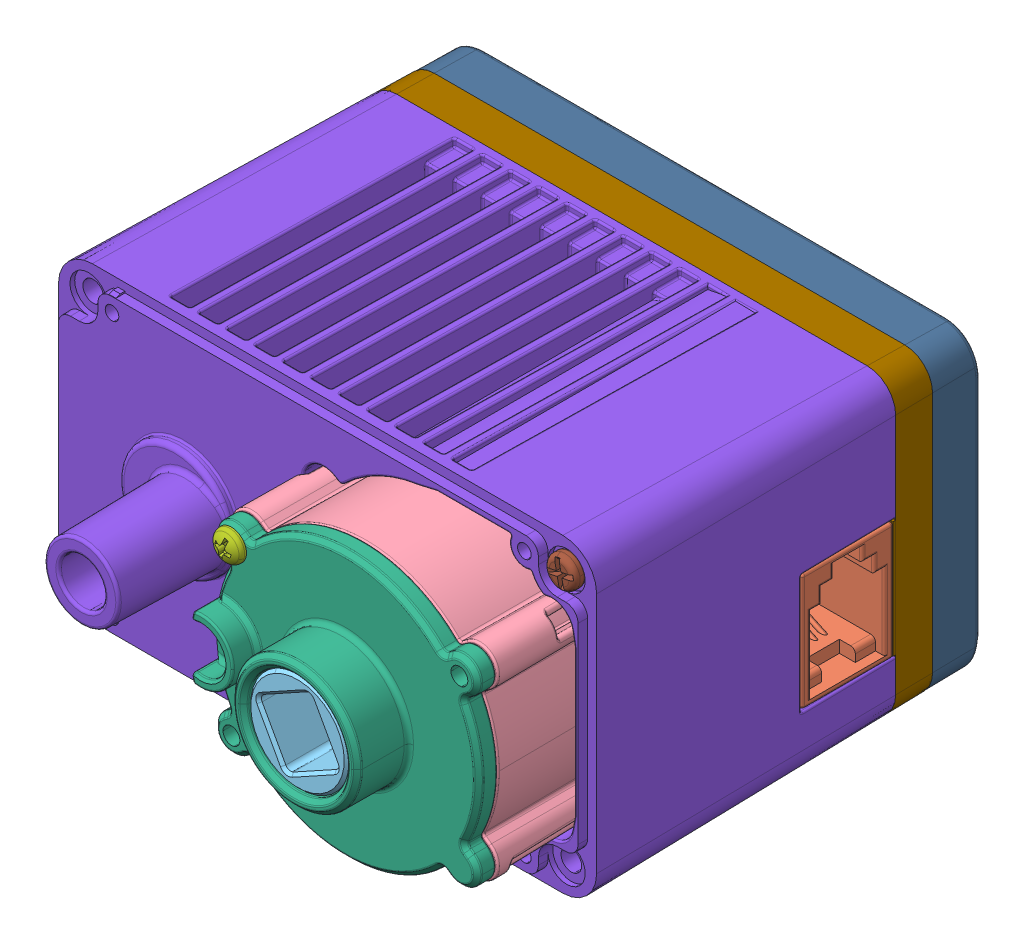
SolidWorks assembly Motor_no_cap_sketch, configuration Default. Lengths in mm.
Overall size (50.17 30.09 0).
20 component instances, 12 part files, 0 mates.
Components (placement in the parent):
- V5 Smart Motor (276-4840).step-1: V5 Smart Motor (276-4840).step [Default] at origin size (59.01 35.33 59.91) (hidden)
  - 276-4840-900 Rev6_Instruction.step-1: 276-4840-900 Rev6_Instruction.step [Default] at (-14.3 0 -17.2) size (52.79 15.94 38.15)
    - 276-4840-901 Rev6.step-1: 276-4840-901 Rev6.step [Default] at (10.75 -10.05 17.8) x (-1 0 0) z (0 0 1) size (49.9 1.6 38.15)
    - 276-4840-902 Rev2.step-1: 276-4840-902 Rev2.step [Default] at (31.25 -9.25 6.2) x (0 0 -1) z (0 -1 0) size (10.35 11.39 15.94)
    - 276-4840-022 Rev4.step-1: 276-4840-022 Rev4.step [Default] at (31.25 -9.25 6.2) x (0 0 -1) z (1 0 0) size (10.26 9.1 5.51)
  - 276-4840-110 Rev10_Instruction.step-1: 276-4840-110 Rev10_Instruction.step [Default] at (12.7 0 14.7) size (35.33 35.33 31.1)
    - 276-4840-061 Rev7_Ring_Gear_Fixed01 .6 Rev3.step-1: 276-4840-061 Rev7_Ring_Gear_Fixed01 .6 Rev3.step [Default] at origin size (28.79 28.39 24.6)
    - 276-4840-018 Rev6.step-1: 276-4840-018 Rev6.step [Default] at (0 0 6.7) x (-0.483174 0.875524 0) z (0 0 1) size (26 26 12.3)
    - 276-4840-059 Rev2.step-1: 276-4840-059 Rev2.step [Default] at (0 0 10.3) size (28.4 28.4 8.5)
    - 276-4840-062 Rev1.step-1: 276-4840-062 Rev1.step [Default] at (-12.1353 8.8168 12.3) x (0.956835 -0.290632 0) z (-0.290632 -0.956835 0) size (3.2 6.56 3.2)
    - 276-4840-062 Rev1.step-2: 276-4840-062 Rev1.step [Default] at (12.1353 8.8168 12.3) x (0.978427 0.206591 0) z (0.206591 -0.978427 0) size (3.2 6.56 3.2)
    - 276-4840-062 Rev1.step-3: 276-4840-062 Rev1.step [Default] at (-12.1353 -8.8168 12.3) x (0.72563 0.688086 0) z (0.688086 -0.72563 0) size (3.2 6.56 3.2)
  - 276-4840-001 Rev38.step-1: 276-4840-001 Rev38.step [Default] at origin size (57.3 33 46.9)
  - 276-4840-005 Rev27.step-1: 276-4840-005 Rev27.step [Default] at (0 0 -17.95) size (56.17 31.87 12.9)
  - 276-4840-004 Rev16.step-1: 276-4840-004 Rev16.step [Default] at (0 0 -19.2) size (56.01 31.71 9.21)
  - 276-4840-009 Rev3.step-1: 276-4840-009 Rev3.step [Default] at (25.45 13.5 15.7) x (0.19987 -0.979823 0) z (-0.979823 -0.19987 0) size (3.4 41.31 4.34)
  - 276-4840-009 Rev3.step-2: 276-4840-009 Rev3.step [Default] at (-25.45 -13.5 15.7) x (-0.998855 0.047836 0) z (0.047836 0.998855 0) size (3.4 41.31 4.34)
  - 276-4840-009 Rev3.step-3: 276-4840-009 Rev3.step [Default] at (25.45 -13.5 15.7) x (-0.975374 0.220559 0) z (0.220559 0.975374 0) size (3.4 41.31 4.34)
  - 276-4840-009 Rev3.step-4: 276-4840-009 Rev3.step [Default] at (-25.45 13.5 15.7) x (-0.922256 0.38658 0) z (0.38658 0.922256 0) size (3.4 41.31 4.34)
  - 276-4840-025 Rev19.step-1: 276-4840-025 Rev19.step [Default] at (12.7 0 -22.63) x (-0.993315 0.115437 0) z (0 0 1) size (14.82 14.83 35.18)
